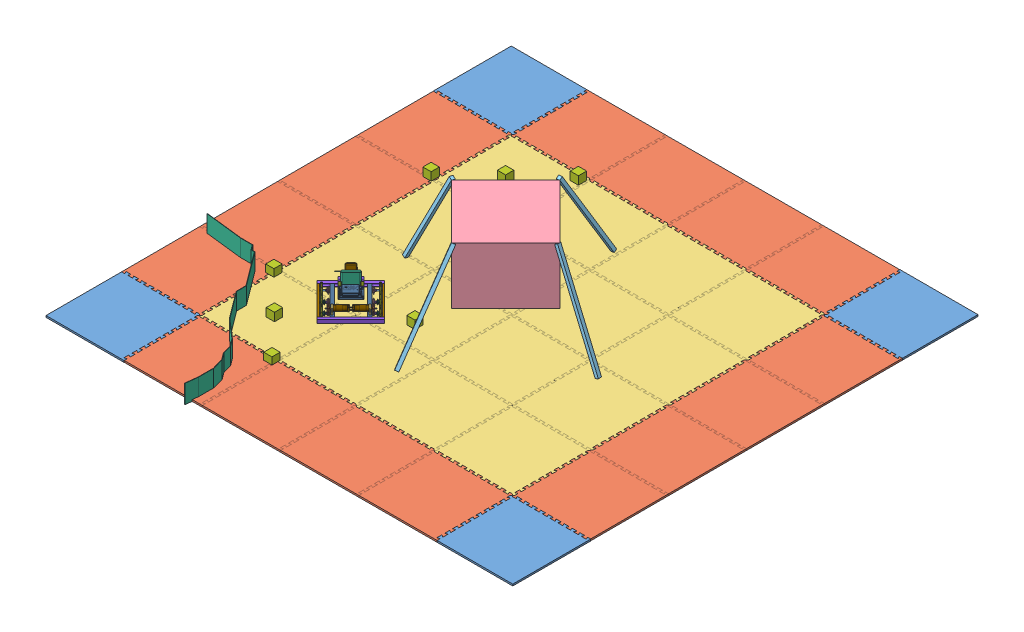
SolidWorks assembly jankfieldlmao, configuration Default. Lengths in mm.
Overall size (3603.71 766.07 3652.23).
154 component instances, 28 part files, 2 mates.
Components (placement in the parent):
- FIELD_RelicRecovery_Tile Field-1: FIELD_RelicRecovery_Tile Field [Default] at (-1722.5806 47.7043 1761.592) size (3603.71 12.7 3603.65)
  - FIELD_RelicRecovery_Corner soft tile-1: FIELD_RelicRecovery_Corner soft tile [Default] at (291.8914 -12.7 -291.8914) size (602.83 12.7 602.83)
  - FIELD_RelicRecovery_Corner soft tile-2: FIELD_RelicRecovery_Corner soft tile [Default] at (3306.0551 -12.7 -297.6546) x (0 0 -1) z (1 0 0) size (602.83 12.7 602.83)
  - FIELD_RelicRecovery_Corner soft tile-3: FIELD_RelicRecovery_Corner soft tile [Default] at (286.1281 -12.7 -3306.0551) x (0 0 1) z (-1 0 0) size (602.83 12.7 602.83)
  - FIELD_RelicRecovery_Corner soft tile-4: FIELD_RelicRecovery_Corner soft tile [Default] at (3300.2918 -12.7 -3311.7596) x (-1 0 0) z (0 0 -1) size (602.83 12.7 602.83)
  - FIELD_RelicRecovery_Side soft tile-1: FIELD_RelicRecovery_Side soft tile [Default] at (894.7241 -12.7 -293.0469) size (621.88 12.7 602.83)
  - FIELD_RelicRecovery_Side soft tile-2: FIELD_RelicRecovery_Side soft tile [Default] at (290.7358 -12.7 -894.7241) x (0 0 1) z (-1 0 0) size (621.88 12.7 602.83)
  - FIELD_RelicRecovery_Side soft tile-3: FIELD_RelicRecovery_Side soft tile [Default] at (1497.5568 -12.7 -294.2025) size (621.88 12.7 602.83)
  - FIELD_RelicRecovery_Side soft tile-4: FIELD_RelicRecovery_Side soft tile [Default] at (2100.3896 -12.7 -295.3581) size (621.88 12.7 602.83)
  - FIELD_RelicRecovery_Side soft tile-5: FIELD_RelicRecovery_Side soft tile [Default] at (2703.2223 -12.7 -296.5137) size (621.88 12.7 602.83)
  - FIELD_RelicRecovery_Side soft tile-6: FIELD_RelicRecovery_Side soft tile [Default] at (289.5802 -12.7 -1497.5568) x (0 0 1) z (-1 0 0) size (621.88 12.7 602.83)
  - FIELD_RelicRecovery_Side soft tile-7: FIELD_RelicRecovery_Side soft tile [Default] at (288.4246 -12.7 -2100.3896) x (0 0 1) z (-1 0 0) size (621.88 12.7 602.83)
  - FIELD_RelicRecovery_Side soft tile-8: FIELD_RelicRecovery_Side soft tile [Default] at (287.2691 -12.7 -2703.2223) x (0 0 1) z (-1 0 0) size (621.88 12.7 602.83)
  - FIELD_RelicRecovery_Side soft tile-9: FIELD_RelicRecovery_Side soft tile [Default] at (888.9609 -12.7 -3307.196) x (-1 0 0) z (0 0 -1) size (621.88 12.7 602.83)
  - FIELD_RelicRecovery_Side soft tile-10: FIELD_RelicRecovery_Side soft tile [Default] at (1491.7936 -12.7 -3308.3369) x (-1 0 0) z (0 0 -1) size (621.88 12.7 602.83)
  - FIELD_RelicRecovery_Side soft tile-11: FIELD_RelicRecovery_Side soft tile [Default] at (2094.6264 -12.7 -3309.4778) x (-1 0 0) z (0 0 -1) size (621.88 12.7 602.83)
  - FIELD_RelicRecovery_Side soft tile-12: FIELD_RelicRecovery_Side soft tile [Default] at (2697.4591 -12.7 -3310.6187) x (-1 0 0) z (0 0 -1) size (621.88 12.7 602.83)
  - FIELD_RelicRecovery_Side soft tile-13: FIELD_RelicRecovery_Side soft tile [Default] at (3301.4327 -12.7 -2708.9269) x (0 0 -1) z (1 0 0) size (621.88 12.7 602.83)
  - FIELD_RelicRecovery_Side soft tile-14: FIELD_RelicRecovery_Side soft tile [Default] at (3302.5737 -12.7 -2106.0942) x (0 0 -1) z (1 0 0) size (621.88 12.7 602.83)
  - FIELD_RelicRecovery_Side soft tile-15: FIELD_RelicRecovery_Side soft tile [Default] at (3303.7146 -12.7 -1503.2614) x (0 0 -1) z (1 0 0) size (621.88 12.7 602.83)
  - FIELD_RelicRecovery_Side soft tile-16: FIELD_RelicRecovery_Side soft tile [Default] at (3304.8555 -12.7 -900.4287) x (0 0 -1) z (1 0 0) size (621.88 12.7 602.83)
  - FIELD_RelicRecovery_Standard soft tile-1: FIELD_RelicRecovery_Standard soft tile [Default] at (893.5685 -12.7 -895.8797) size (621.88 12.7 621.88)
  - FIELD_RelicRecovery_Standard soft tile-2: FIELD_RelicRecovery_Standard soft tile [Default] at (892.413 -12.7 -1498.7124) size (621.88 12.7 621.88)
  - FIELD_RelicRecovery_Standard soft tile-3: FIELD_RelicRecovery_Standard soft tile [Default] at (891.2574 -12.7 -2101.5452) size (621.88 12.7 621.88)
  - FIELD_RelicRecovery_Standard soft tile-4: FIELD_RelicRecovery_Standard soft tile [Default] at (890.1018 -12.7 -2704.3779) size (621.88 12.7 621.88)
  - FIELD_RelicRecovery_Standard soft tile-5: FIELD_RelicRecovery_Standard soft tile [Default] at (1496.4013 -12.7 -897.0353) size (621.88 12.7 621.88)
  - FIELD_RelicRecovery_Standard soft tile-6: FIELD_RelicRecovery_Standard soft tile [Default] at (1495.2457 -12.7 -1499.868) size (621.88 12.7 621.88)
  - FIELD_RelicRecovery_Standard soft tile-7: FIELD_RelicRecovery_Standard soft tile [Default] at (1494.0901 -12.7 -2102.7007) size (621.88 12.7 621.88)
  - FIELD_RelicRecovery_Standard soft tile-8: FIELD_RelicRecovery_Standard soft tile [Default] at (1492.9345 -12.7 -2705.5335) size (621.88 12.7 621.88)
  - FIELD_RelicRecovery_Standard soft tile-9: FIELD_RelicRecovery_Standard soft tile [Default] at (2099.234 -12.7 -898.1908) size (621.88 12.7 621.88)
  - FIELD_RelicRecovery_Standard soft tile-10: FIELD_RelicRecovery_Standard soft tile [Default] at (2098.0784 -12.7 -1501.0236) size (621.88 12.7 621.88)
  - FIELD_RelicRecovery_Standard soft tile-11: FIELD_RelicRecovery_Standard soft tile [Default] at (2096.9228 -12.7 -2103.8563) size (621.88 12.7 621.88)
  - FIELD_RelicRecovery_Standard soft tile-12: FIELD_RelicRecovery_Standard soft tile [Default] at (2095.7673 -12.7 -2706.689) size (621.88 12.7 621.88)
  - FIELD_RelicRecovery_Standard soft tile-13: FIELD_RelicRecovery_Standard soft tile [Default] at (2702.0667 -12.7 -899.3464) size (621.88 12.7 621.88)
  - FIELD_RelicRecovery_Standard soft tile-14: FIELD_RelicRecovery_Standard soft tile [Default] at (2700.9112 -12.7 -1502.1791) size (621.88 12.7 621.88)
  - FIELD_RelicRecovery_Standard soft tile-15: FIELD_RelicRecovery_Standard soft tile [Default] at (2699.7556 -12.7 -2105.0119) size (621.88 12.7 621.88)
  - FIELD_RelicRecovery_Standard soft tile-16: FIELD_RelicRecovery_Standard soft tile [Default] at (2698.6 -12.7 -2707.8446) size (621.88 12.7 621.88)
- Assem1-1: Assem1 [Default] at (-345.7098 170.5102 -63.598) x (0.707107 0 -0.707107) z (0.707107 0 0.707107) size (1212.6 747.66 1171.24)
  - landerBody-1: landerBody [Default] at (321.6828 178.1754 363.226) size (591.82 439.42 591.82)
  - landerLegs-1: landerLegs [Default] at (757.5041 -108.5653 925.7867) x (-0.665044 -0.418518 -0.618514) z (0.692784 -0.036473 -0.720222) size (25.4 797.56 25.4)
  - landerLegs-2: landerLegs [Default] at (833.0645 -63.9982 -208.5204) x (0.534547 0.510671 -0.673406) z (0.758575 0.061365 0.64869) size (25.4 797.56 25.4)
  - landerLegs-3: landerLegs [Default] at (-342.3782 -98.5367 874.384) x (-0.919891 0.356278 -0.163912) z (0.051837 -0.303829 -0.951315) size (25.4 797.56 25.4)
  - landerLegs-4: landerLegs [Default] at (-306.2525 -82.7813 -199.247) x (0.456169 -0.450226 0.767598) z (-0.830357 0.094851 0.5491) size (25.4 797.56 25.4)
- crter lol-1: crter lol [Default] at (-875.4653 178.5063 970.4536) size (1061.15 143 1222.76)
- gold-1: gold [Default] at (-1161.7992 41.3904 615.4522) size (63.5 63.5 63.5)
- gold-2: gold [Default] at (-861.9809 47.7043 911.0218) size (63.5 63.5 63.5)
- gold-3: gold [Default] at (-582.5643 38.5098 1209.8894) size (63.5 63.5 63.5)
- CH_ASSEM_FULL-2: CH_ASSEM_FULL [Default] at (-803.1989 -47.8095 473.1309) x (0.707107 0 -0.707107) z (0.707107 0 0.707107) size (404.11 208.98 368.3)
  - CH_ASSEM_Base-1: CH_ASSEM_Base [Default] at (-90.7761 -10.2499 -116.5851) size (368.3 25.4 368.3)
    - CH_FrontBackChannel-2: CH_FrontBackChannel [Default] at (378.7562 204.4057 248.334) x (0 1 0) z (0 0 1) size (25.4 368.3 25.4)
    - CH_SideOuterChannel-2: CH_SideOuterChannel [Default] at (23.1562 207.5807 226.109) x (0 1 0) z (1 0 0) size (19.05 361.95 12.7)
    - CH_FrontBackChannel-3: CH_FrontBackChannel [Default] at (378.7562 229.8057 565.834) x (0 -1 0) z (0 0 -1) size (25.4 368.3 25.4)
    - CH_SideInnerChannel-3: CH_SideInnerChannel [Default] at (80.0522 207.5807 588.059) x (0 1 0) z (-1 0 0) size (19.05 361.95 25.4)
    - CH_SideInnerChannel-4: CH_SideInnerChannel [Default] at (309.1602 226.6307 588.059) x (0 -1 0) z (1 0 0) size (19.05 361.95 25.4)
    - CH_SideOuterChannel-5: CH_SideOuterChannel [Default] at (366.0562 226.6307 226.109) x (0 -1 0) z (-1 0 0) size (19.05 361.95 12.7)
  - CH_ASSEM_DriveWheel-1: CH_ASSEM_DriveWheel [Default] at (59.5626 215.0895 411.9658) x (0 0 1) z (-1 0 0) size (123.02 123.02 97.03)
    - CH_ASSEM_BearingBlock-1: CH_ASSEM_BearingBlock [Default] at (2.3581 -14.5837 48.57) size (29.51 14.04 11.53)
      - PART_BearingBlock-1: PART_BearingBlock [Default] at (-29.5139 0 12.1915) x (1 0 0) z (0 -1 0) size (29.51 9.53 12.7)
      - PART_BearingThroughBoreLong-1: PART_BearingThroughBoreLong [Default] at (-14.7569 7.5406 21.7165) size (13 13 11)
    - CH_ASSEM_DriveWheelShaft-1: CH_ASSEM_DriveWheelShaft [Default] at (-19.3547 -19.6717 70.3125) x (0.866025 -0.5 0) z (0 0 1) size (90.05 90.05 96.5)
      - PART_Gear30Tooth-1: PART_Gear30Tooth [Default] at (-0.2904 14.4147 9.474) size (24.32 24.24 15)
      - PART_HexShaft75mm-1: PART_HexShaft75mm [Default] at (-0.2904 14.4147 -9.026) size (5 5.77 75)
      - PART_Sprocket15Tooth-1: PART_Sprocket15Tooth [Default] at (-0.2904 14.4147 32.474) size (33.59 33.42 15)
      - PART_TractionWheel90mm-1: PART_TractionWheel90mm [Default] at (-0.2904 14.4147 47.474) size (90.05 90.05 80)
      - PART_ShaftCollar-1: PART_ShaftCollar [Default] at (-0.2904 14.4147 20.974) size (13 13 8)
    - CH_ASSEM_BearingBlock-2: CH_ASSEM_BearingBlock [Default] at (-27.1558 -14.5837 149.0031) x (-1 0 0) z (0 0 -1) size (29.51 14.04 11.53)
      - PART_BearingBlock-1: PART_BearingBlock [Default] at (-29.5139 0 12.1915) x (1 0 0) z (0 -1 0) size (29.51 9.53 12.7)
      - PART_BearingThroughBoreLong-1: PART_BearingThroughBoreLong [Default] at (-14.7569 7.5406 21.7165) size (13 13 11)
  - PART_ASSEM_MotorHDHexRotating-1: PART_ASSEM_MotorHDHexRotating [Default] at (134.2476 254.6096 293.9221) x (0 -0.92311 0.384536) z (-1 0 0) size (38 39.44 154.16)
    - PART_MotorHDHex_Shell-1: PART_MotorHDHex_Shell [Default] at (52.6409 85.4657 114.2715) size (38 39.44 128.25)
    - PART_MotorHDHex_RotatingHex-1: PART_MotorHDHex_RotatingHex [Default] at (52.6787 94.995 172.8795) x (0.858442 -0.512911 0) z (0.512911 0.858442 0) size (5.06 33.53 5.84)
  - PART_Gear60Tooth-1: PART_Gear60Tooth [Default] at (-20.2239 241.5359 399.567) x (0 0.989669 0.143372) z (1 0 0) size (47.04 47.04 15)
  - PART_MotorMount-1: PART_MotorMount [Default] at (6.2756 238.7668 404.1993) x (0 0 -1) z (1 0 0) size (72 44.98 12.7)
  - CH_Assem_CentreWheel-1: CH_Assem_CentreWheel [Default] at (2.6857 228.0574 315.7728) x (0 0 -1) z (-1 0 0) size (123.02 123.02 97.03)
    - CH_ASSEM_BearingBlock-1: CH_ASSEM_BearingBlock [Default] at (40.0308 14.8515 -8.3069) size (29.51 14.04 11.53)
      - PART_BearingBlock-1: PART_BearingBlock [Default] at (-29.5139 0 12.1915) x (1 0 0) z (0 -1 0) size (29.51 9.53 12.7)
      - PART_BearingThroughBoreLong-1: PART_BearingThroughBoreLong [Default] at (-14.7569 7.5406 21.7165) size (13 13 11)
    - CH_Assem_CentreWheelShaft-1: CH_Assem_CentreWheelShaft [Default] at (67.892 -5.5775 97.812) x (-0.866025 -0.5 0) z (0 0 -1) size (90.05 90.05 96.5)
      - PART_HexShaft75mm-1: PART_HexShaft75mm [Default] at (22.9236 45.5315 18.4024) size (5 5.77 75)
      - PART_Sprocket15Tooth-1: PART_Sprocket15Tooth [Default] at (22.9236 45.5315 51.9024) size (33.59 33.42 15)
      - PART_Sprocket20Tooth-1: PART_Sprocket20Tooth [Default] at (22.9236 45.5315 74.9024) size (43.5 43.5 15)
      - PART_TractionWheel90mm-1: PART_TractionWheel90mm [Default] at (22.9236 45.5315 36.9024) size (90.05 90.05 80)
      - PART_ShaftCollar-1: PART_ShaftCollar [Default] at (22.9236 45.5315 63.4024) size (13 13 8)
    - CH_ASSEM_BearingBlock-2: CH_ASSEM_BearingBlock [Default] at (10.5169 14.8515 92.1262) x (-1 0 0) z (0 0 -1) size (29.51 14.04 11.53)
      - PART_BearingBlock-1: PART_BearingBlock [Default] at (-29.5139 0 12.1915) x (1 0 0) z (0 -1 0) size (29.51 9.53 12.7)
      - PART_BearingThroughBoreLong-1: PART_BearingThroughBoreLong [Default] at (-14.7569 7.5406 21.7165) size (13 13 11)
  - CH_ASSEM_EndWheel-1: CH_ASSEM_EndWheel [Default] at (-69.5235 200.5058 196.1878) x (0 0 1) z (-1 0 0) size (123.02 123.02 97.03)
    - CH_ASSEM_BearingBlock-1: CH_ASSEM_BearingBlock [Default] at (0 0 -80.5161) size (29.51 14.04 11.53)
      - PART_BearingBlock-1: PART_BearingBlock [Default] at (-29.5139 0 12.1915) x (1 0 0) z (0 -1 0) size (29.51 9.53 12.7)
      - PART_BearingThroughBoreLong-1: PART_BearingThroughBoreLong [Default] at (-14.7569 7.5406 21.7165) size (13 13 11)
    - CH_ASSEM_EndWheelShaft-1: CH_ASSEM_EndWheelShaft [Default] at (-15.9553 -39.3245 28.8345) x (-0.866025 0.5 0) z (0 0 -1) size (90.05 90.05 96.5)
      - PART_HexShaft75mm-1: PART_HexShaft75mm [Default] at (22.3948 41.1855 21.634) size (5 5.77 75)
      - PART_Spacer15mm-1: PART_Spacer15mm [Default] at (22.3948 41.1855 55.134) size (8.79 8.79 15)
      - PART_Sprocket20Tooth-1: PART_Sprocket20Tooth [Default] at (22.3948 41.1855 78.134) size (43.5 43.5 15)
      - PART_TractionWheel90mm-1: PART_TractionWheel90mm [Default] at (22.3948 41.1855 40.134) size (90.05 90.05 80)
      - PART_ShaftCollar-1: PART_ShaftCollar [Default] at (22.3948 41.1855 66.634) size (13 13 8)
    - CH_ASSEM_BearingBlock-2: CH_ASSEM_BearingBlock [Default] at (-29.5139 0 19.917) x (-1 0 0) z (0 0 -1) size (29.51 14.04 11.53)
      - PART_BearingBlock-1: PART_BearingBlock [Default] at (-29.5139 0 12.1915) x (1 0 0) z (0 -1 0) size (29.51 9.53 12.7)
      - PART_BearingThroughBoreLong-1: PART_BearingThroughBoreLong [Default] at (-14.7569 7.5406 21.7165) size (13 13 11)
  - PART_ASSEM_MotorHDHexRotating-2: PART_ASSEM_MotorHDHexRotating [Default] at (73.4126 157.4229 334.4067) x (0 0.92311 -0.384536) z (1 0 0) size (38 39.44 154.16)
    - PART_MotorHDHex_Shell-1: PART_MotorHDHex_Shell [Default] at (52.6409 85.4657 114.2715) size (38 39.44 128.25)
    - PART_MotorHDHex_RotatingHex-1: PART_MotorHDHex_RotatingHex [Default] at (52.6787 94.995 172.8795) x (0.858442 -0.512911 0) z (0.512911 0.858442 0) size (5.06 33.53 5.84)
  - CH_ASSEM_DriveWheel-2: CH_ASSEM_DriveWheel [Default] at (148.0976 215.0895 387.1681) x (0 0 -1) z (1 0 0) size (123.02 123.02 97.03)
    - CH_ASSEM_BearingBlock-1: CH_ASSEM_BearingBlock [Default] at (2.3581 -14.5837 48.57) size (29.51 14.04 11.53)
      - PART_BearingBlock-1: PART_BearingBlock [Default] at (-29.5139 0 12.1915) x (1 0 0) z (0 -1 0) size (29.51 9.53 12.7)
      - PART_BearingThroughBoreLong-1: PART_BearingThroughBoreLong [Default] at (-14.7569 7.5406 21.7165) size (13 13 11)
    - CH_ASSEM_DriveWheelShaft-1: CH_ASSEM_DriveWheelShaft [Default] at (-19.3547 -19.6717 70.3125) x (0.866025 -0.5 0) z (0 0 1) size (90.05 90.05 96.5)
      - PART_Gear30Tooth-1: PART_Gear30Tooth [Default] at (-0.2904 14.4147 9.474) size (24.32 24.24 15)
      - PART_HexShaft75mm-1: PART_HexShaft75mm [Default] at (-0.2904 14.4147 -9.026) size (5 5.77 75)
      - PART_Sprocket15Tooth-1: PART_Sprocket15Tooth [Default] at (-0.2904 14.4147 32.474) size (33.59 33.42 15)
      - PART_TractionWheel90mm-1: PART_TractionWheel90mm [Default] at (-0.2904 14.4147 47.474) size (90.05 90.05 80)
      - PART_ShaftCollar-1: PART_ShaftCollar [Default] at (-0.2904 14.4147 20.974) size (13 13 8)
    - CH_ASSEM_BearingBlock-2: CH_ASSEM_BearingBlock [Default] at (-27.1558 -14.5837 149.0031) x (-1 0 0) z (0 0 -1) size (29.51 14.04 11.53)
      - PART_BearingBlock-1: PART_BearingBlock [Default] at (-29.5139 0 12.1915) x (1 0 0) z (0 -1 0) size (29.51 9.53 12.7)
      - PART_BearingThroughBoreLong-1: PART_BearingThroughBoreLong [Default] at (-14.7569 7.5406 21.7165) size (13 13 11)
  - PART_Gear60Tooth-2: PART_Gear60Tooth [Default] at (227.8841 241.5359 399.567) x (0 -0.989669 -0.143372) z (-1 0 0) size (47.04 47.04 15)
  - PART_MotorMount-2: PART_MotorMount [Default] at (213.2836 238.7668 404.1993) x (0 0 -1) z (1 0 0) size (72 44.98 12.7)
  - CH_Assem_CentreWheel-2: CH_Assem_CentreWheel [Default] at (204.9745 228.0574 265.2251) x (0 0 1) z (1 0 0) size (123.02 123.02 97.03)
    - CH_ASSEM_BearingBlock-1: CH_ASSEM_BearingBlock [Default] at (40.0308 14.8515 -8.3069) size (29.51 14.04 11.53)
      - PART_BearingBlock-1: PART_BearingBlock [Default] at (-29.5139 0 12.1915) x (1 0 0) z (0 -1 0) size (29.51 9.53 12.7)
      - PART_BearingThroughBoreLong-1: PART_BearingThroughBoreLong [Default] at (-14.7569 7.5406 21.7165) size (13 13 11)
    - CH_Assem_CentreWheelShaft-1: CH_Assem_CentreWheelShaft [Default] at (67.892 -5.5775 97.812) x (-0.866025 -0.5 0) z (0 0 -1) size (90.05 90.05 96.5)
      - PART_HexShaft75mm-1: PART_HexShaft75mm [Default] at (22.9236 45.5315 18.4024) size (5 5.77 75)
      - PART_Sprocket15Tooth-1: PART_Sprocket15Tooth [Default] at (22.9236 45.5315 51.9024) size (33.59 33.42 15)
      - PART_Sprocket20Tooth-1: PART_Sprocket20Tooth [Default] at (22.9236 45.5315 74.9024) size (43.5 43.5 15)
      - PART_TractionWheel90mm-1: PART_TractionWheel90mm [Default] at (22.9236 45.5315 36.9024) size (90.05 90.05 80)
      - PART_ShaftCollar-1: PART_ShaftCollar [Default] at (22.9236 45.5315 63.4024) size (13 13 8)
    - CH_ASSEM_BearingBlock-2: CH_ASSEM_BearingBlock [Default] at (10.5169 14.8515 92.1262) x (-1 0 0) z (0 0 -1) size (29.51 14.04 11.53)
      - PART_BearingBlock-1: PART_BearingBlock [Default] at (-29.5139 0 12.1915) x (1 0 0) z (0 -1 0) size (29.51 9.53 12.7)
      - PART_BearingThroughBoreLong-1: PART_BearingThroughBoreLong [Default] at (-14.7569 7.5406 21.7165) size (13 13 11)
  - CH_ASSEM_EndWheel-2: CH_ASSEM_EndWheel [Default] at (277.1837 215.5871 196.1878) x (0 0 1) z (1 0 0) size (123.02 123.02 97.03)
    - CH_ASSEM_BearingBlock-1: CH_ASSEM_BearingBlock [Default] at (0 0 -80.5161) size (29.51 14.04 11.53)
      - PART_BearingBlock-1: PART_BearingBlock [Default] at (-29.5139 0 12.1915) x (1 0 0) z (0 -1 0) size (29.51 9.53 12.7)
      - PART_BearingThroughBoreLong-1: PART_BearingThroughBoreLong [Default] at (-14.7569 7.5406 21.7165) size (13 13 11)
    - CH_ASSEM_EndWheelShaft-1: CH_ASSEM_EndWheelShaft [Default] at (-15.9553 -39.3245 28.8345) x (-0.866025 0.5 0) z (0 0 -1) size (90.05 90.05 96.5)
      - PART_HexShaft75mm-1: PART_HexShaft75mm [Default] at (22.3948 41.1855 21.634) size (5 5.77 75)
      - PART_Spacer15mm-1: PART_Spacer15mm [Default] at (22.3948 41.1855 55.134) size (8.79 8.79 15)
      - PART_Sprocket20Tooth-1: PART_Sprocket20Tooth [Default] at (22.3948 41.1855 78.134) size (43.5 43.5 15)
      - PART_TractionWheel90mm-1: PART_TractionWheel90mm [Default] at (22.3948 41.1855 40.134) size (90.05 90.05 80)
      - PART_ShaftCollar-1: PART_ShaftCollar [Default] at (22.3948 41.1855 66.634) size (13 13 8)
    - CH_ASSEM_BearingBlock-2: CH_ASSEM_BearingBlock [Default] at (-29.5139 0 19.917) x (-1 0 0) z (0 0 -1) size (29.51 14.04 11.53)
      - PART_BearingBlock-1: PART_BearingBlock [Default] at (-29.5139 0 12.1915) x (1 0 0) z (0 -1 0) size (29.51 9.53 12.7)
      - PART_BearingThroughBoreLong-1: PART_BearingThroughBoreLong [Default] at (-14.7569 7.5406 21.7165) size (13 13 11)
  - CH_ASSEM_BatteryPhone-1: CH_ASSEM_BatteryPhone [Default] at (39.7502 187.7674 170.7548) x (0 0 -1) z (1 0 0) size (44.45 133.58 161.51)
    - PART_BatterySlim12V-1: PART_BatterySlim12V [Default] at (26.3058 77.0384 64.08) x (0 -1 0) z (0 0 1) size (90.56 23.03 147.25)
    - PART_SlimBatteryClip-1: PART_SlimBatteryClip [Default] at (39.0058 31.7884 107.3076) x (0 0 -1) z (1 0 0) size (18.01 28.57 25.4)
    - PART_SlimBatteryClip-2: PART_SlimBatteryClip [Default] at (13.6058 31.7884 20.8523) x (0 0 1) z (-1 0 0) size (18.01 28.57 25.4)
    - PART_PhoneSupportSheet-1: PART_PhoneSupportSheet [Default] at (58.0558 60.3634 134.692) x (0 0 -1) z (1 0 0) size (141.22 3.17 44.45)
    - PART_ZTESpeed-1: PART_ZTESpeed [Default] at (40.0121 98.6181 70.154) x (0 0 1) z (-1 0 0) size (68.17 133.58 10.49)
  - PART_ExpansionHub-1: PART_ExpansionHub [Default] at (103.8301 219.4847 232.4629) x (0 0 1) z (-1 0 0) size (103 29.58 143)
- gold-4: gold [Default] at (-267.4187 47.7043 420.6725) size (63.5 63.5 63.5)
- gold-5: gold [Default] at (-580.6711 68.4118 -1154.3556) size (63.5 63.5 63.5)
- gold-6: gold [Default] at (-867.4446 68.4118 -878.7352) size (63.5 63.5 63.5)
- gold-7: gold [Default] at (-1176.4284 68.4118 -612.7612) size (63.5 63.5 63.5)
Mates (geometry in assembly coordinates):
- Coincident2: coincident anti-aligned: plane of FIELD_RelicRecovery_Tile Field-1/FIELD_RelicRecovery_Standard soft tile-1 through (-829.0121 47.7043 865.7123) normal (0 1 0); plane of gold-2 through (-861.9809 47.7043 911.0218) normal (0 -1 0)
- Coincident3: coincident: plane of FIELD_RelicRecovery_Tile Field-1/FIELD_RelicRecovery_Standard soft tile-6 through (-227.3349 47.7043 261.724) normal (0 1 0); line of gold-4 through (-203.9187 47.7043 431.3857) axis (0 0 -1)
